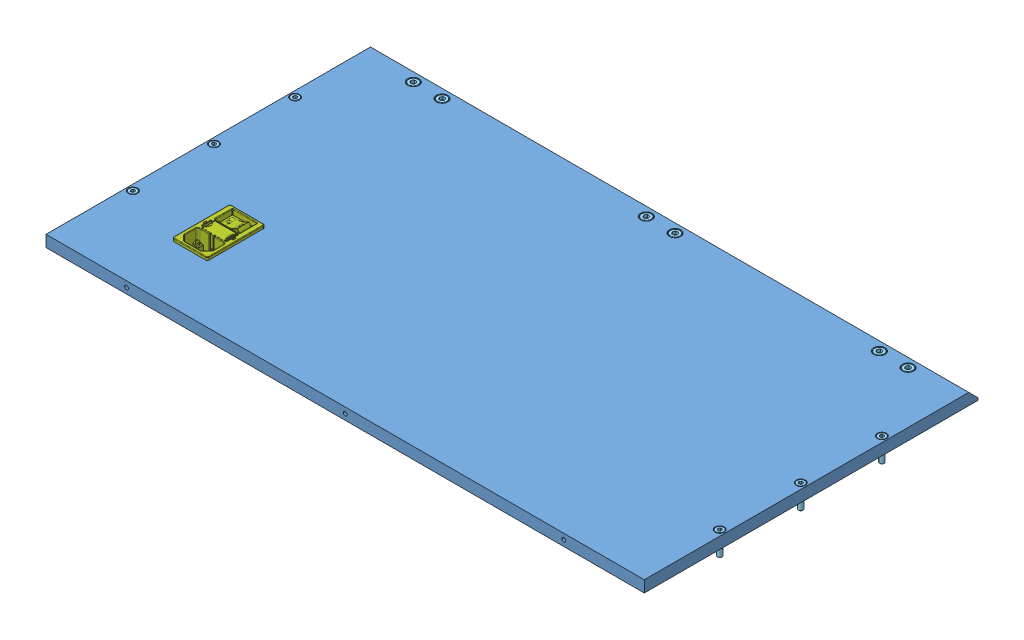
SolidWorks assembly Housing_back, configuration Default. Lengths in mm.
Overall size (520 63.66 290).
37 component instances, 9 part files, 59 mates.
Components (placement in the parent):
- Housing_back-1: Housing_back [Default] at origin size (520 10 290)
- SHPSNA5-1: SHPSNA5 [Closed] at (223 -4.6 -284.75) x (0 0 -1) z (-1 0 0) size (23.16 23.61 41)
  - SHPSNA5_3-1: SHPSNA5_3 [Default] at origin size (22.6 9.2 41)
  - SHPSNA5_7-1: SHPSNA5_7 [Default] x (-0.41399 -0.910281 0) z (0 0 1) size (5 5 41)
  - SHPSNA5_5-1: SHPSNA5_5 [Default] x (-0.130353 0.991468 0) z (0 0 1) size (22.6 9.2 41)
- SHPSNA5-2: SHPSNA5 [Closed] at (20.5 -4.6 -284.75) x (0 0 -1) z (-1 0 0) size (23.16 23.61 41)
  - SHPSNA5_3-1: SHPSNA5_3 [Default] at origin size (22.6 9.2 41)
  - SHPSNA5_7-1: SHPSNA5_7 [Default] x (-0.41399 -0.910281 0) z (0 0 1) size (5 5 41)
  - SHPSNA5_5-1: SHPSNA5_5 [Default] x (-0.130353 0.991468 0) z (0 0 1) size (22.6 9.2 41)
- SHPSNA5-3: SHPSNA5 [Closed] at (-182 -4.6 -284.75) x (0 0 -1) z (-1 0 0) size (23.16 23.61 41)
  - SHPSNA5_3-1: SHPSNA5_3 [Default] at origin size (22.6 9.2 41)
  - SHPSNA5_7-1: SHPSNA5_7 [Default] x (-0.41399 -0.910281 0) z (0 0 1) size (5 5 41)
  - SHPSNA5_5-1: SHPSNA5_5 [Default] x (-0.130353 0.991468 0) z (0 0 1) size (22.6 9.2 41)
- socket head cap screw_iso-2: socket head cap screw_iso [ISO 4762 M5 x 10 - 10N] at (-215 10 -274.25) x (0 -1 0) z (0 0 1) size (15 8.5 8.5)
- socket head cap screw_iso-3: socket head cap screw_iso [ISO 4762 M5 x 10 - 10N] at (-190 10 -274.25) x (0 -1 0) z (0 0 1) size (15 8.5 8.5)
- socket head cap screw_iso-4: socket head cap screw_iso [ISO 4762 M5 x 10 - 10N] at (-12.5 10 -274.25) x (0 -1 0) z (0 0 1) size (15 8.5 8.5)
- socket head cap screw_iso-5: socket head cap screw_iso [ISO 4762 M5 x 10 - 10N] at (12.5 10 -274.25) x (0 -1 0) z (0 0 1) size (15 8.5 8.5)
- socket head cap screw_iso-6: socket head cap screw_iso [ISO 4762 M5 x 10 - 10N] at (190 10 -274.25) x (0 -1 0) z (0 0 1) size (15 8.5 8.5)
- socket head cap screw_iso-7: socket head cap screw_iso [ISO 4762 M5 x 10 - 10N] at (215 10 -274.25) x (0 -1 0) z (0 0 1) size (15 8.5 8.5)
- hex thin nut gradeb_iso-2: hex thin nut gradeb_iso [ISO - 4036 - M5 - N] at (215 -4.7 -274.25) x (1 0 0) z (0 -1 0) size (8 9.24 2.7)
- hex thin nut gradeb_iso-3: hex thin nut gradeb_iso [ISO - 4036 - M5 - N] at (190 -4.7 -274.25) x (1 0 0) z (0 -1 0) size (8 9.24 2.7)
- hex thin nut gradeb_iso-4: hex thin nut gradeb_iso [ISO - 4036 - M5 - N] at (12.5 -4.7 -274.25) x (1 0 0) z (0 -1 0) size (8 9.24 2.7)
- hex thin nut gradeb_iso-5: hex thin nut gradeb_iso [ISO - 4036 - M5 - N] at (-12.5 -4.7 -274.25) x (1 0 0) z (0 -1 0) size (8 9.24 2.7)
- hex thin nut gradeb_iso-6: hex thin nut gradeb_iso [ISO - 4036 - M5 - N] at (-190 -4.7 -274.25) x (1 0 0) z (0 -1 0) size (8 9.24 2.7)
- hex thin nut gradeb_iso-7: hex thin nut gradeb_iso [ISO - 4036 - M5 - N] at (-215 -4.7 -274.25) x (1 0 0) z (0 -1 0) size (8 9.24 2.7)
- socket head cap screw_iso-9: socket head cap screw_iso [ISO 4762 M4 x 16 - 16N] at (-255 10 -211.5) x (0 -1 0) z (0 0 1) size (20 7 7)
- socket head cap screw_iso-10: socket head cap screw_iso [ISO 4762 M4 x 16 - 16N] at (-255 10 -141) x (0 -1 0) z (0 0 1) size (20 7 7)
- socket head cap screw_iso-11: socket head cap screw_iso [ISO 4762 M4 x 16 - 16N] at (-255 10 -70.5) x (0 -1 0) z (0 0 1) size (20 7 7)
- socket head cap screw_iso-12: socket head cap screw_iso [ISO 4762 M4 x 16 - 16N] at (255 10 -70.5) x (0 -1 0) z (0 0 1) size (20 7 7)
- socket head cap screw_iso-13: socket head cap screw_iso [ISO 4762 M4 x 16 - 16N] at (255 10 -211.5) x (0 -1 0) z (0 0 1) size (20 7 7)
- socket head cap screw_iso-14: socket head cap screw_iso [ISO 4762 M4 x 16 - 16N] at (255 10 -141) x (0 -1 0) z (0 0 1) size (20 7 7)
- KMF1.1291.11-1: KMF1.1291.11 [Default] at (-185 10 -60.7) x (-1 0 0) z (0 -1 0) size (31.8 50 43.41)
- CUS-150M-F-1: CUS-150M-F [Default] at (-121.4398 -2.8109 -148.4745) x (0.999999 0 0.001586) z (0.001586 0 -0.999999) size (116.08 50.7 64.1)
- pan head cross recess screw_iso-1: pan head cross recess screw_iso [ISO 7045 - M4 x 6 - Z - 6N] at (-210 -4.3 -140) x (0 1 0) z (-0.546944 0 0.837169) size (9.02 8 8)
- pan head cross recess screw_iso-2: pan head cross recess screw_iso [ISO 7045 - M4 x 6 - Z - 6N] at (-210 -4.3 -175) x (0 1 0) z (-0.546944 0 0.837169) size (9.02 8 8)
- pan head cross recess screw_iso-3: pan head cross recess screw_iso [ISO 7045 - M4 x 6 - Z - 6N] at (-99.4 -4.3 -140) x (0 1 0) z (-0.546944 0 0.837169) size (9.02 8 8)
- pan head cross recess screw_iso-4: pan head cross recess screw_iso [ISO 7045 - M4 x 6 - Z - 6N] at (-99.4 -4.3 -175) x (0 1 0) z (-0.546944 0 0.837169) size (9.02 8 8)
Mates (geometry in assembly coordinates):
- Coincident1: coincident anti-aligned: plane of Housing_back-1 through (0 0 0) normal (0 -1 0); plane of SHPSNA5-1/SHPSNA5_3-1 through (182 0 -266.75) normal (0 1 0)
- Coincident3: coincident anti-aligned: plane of Housing_back-1 through (0 0 0) normal (0 -1 0); plane of SHPSNA5-2/SHPSNA5_3-1 through (-20.5 0 -266.75) normal (0 1 0)
- Coincident4: coincident anti-aligned: plane of Housing_back-1 through (0 0 0) normal (0 -1 0); plane of SHPSNA5-3/SHPSNA5_3-1 through (-223 0 -266.75) normal (0 1 0)
- Concentric1: concentric aligned: cylinder of Housing_back-1 through (-215 10 -274.25) axis (0 1 0) radius 5; cylinder of SHPSNA5-3/SHPSNA5_3-1 through (-215 -2 -274.25) axis (0 1 0) radius 2.75
- Concentric2: concentric aligned: cylinder of Housing_back-1 through (-190 10 -274.25) axis (0 1 0) radius 5; cylinder of SHPSNA5-3/SHPSNA5_3-1 through (-190 -2 -274.25) axis (0 1 0) radius 2.75
- Concentric3: concentric aligned: cylinder of Housing_back-1 through (-12.5 10 -274.25) axis (0 1 0) radius 5; cylinder of SHPSNA5-2/SHPSNA5_3-1 through (-12.5 -2 -274.25) axis (0 1 0) radius 2.75
- Concentric4: concentric aligned: cylinder of Housing_back-1 through (12.5 10 -274.25) axis (0 1 0) radius 5; cylinder of SHPSNA5-2/SHPSNA5_3-1 through (12.5 -2 -274.25) axis (0 1 0) radius 2.75
- Concentric5: concentric aligned: cylinder of Housing_back-1 through (190 10 -274.25) axis (0 1 0) radius 5; cylinder of SHPSNA5-1/SHPSNA5_3-1 through (190 -2 -274.25) axis (0 1 0) radius 2.75
- Concentric6: concentric aligned: cylinder of Housing_back-1 through (215 10 -274.25) axis (0 1 0) radius 5; cylinder of SHPSNA5-1/SHPSNA5_3-1 through (215 -2 -274.25) axis (0 1 0) radius 2.75
- Concentric7: concentric aligned: cylinder of Housing_back-1 through (-215 10 -274.25) axis (0 1 0) radius 2.75; cylinder of socket head cap screw_iso-2 through (-215 41.75 -274.25) axis (0 1 0) radius 4.25
- Coincident5: coincident anti-aligned: plane of Housing_back-1 through (-212.25 5 -274.25) normal (0 1 0); plane of socket head cap screw_iso-2 through (-210.75 5 -274.25) normal (0 -1 0)
- Concentric8: concentric aligned: cylinder of Housing_back-1 through (-190 10 -274.25) axis (0 1 0) radius 5; cylinder of socket head cap screw_iso-3 through (-190 41.75 -274.25) axis (0 1 0) radius 4.25
- Coincident6: coincident anti-aligned: plane of Housing_back-1 through (-187.25 5 -274.25) normal (0 1 0); plane of socket head cap screw_iso-3 through (-185.75 5 -274.25) normal (0 -1 0)
- Concentric9: concentric aligned: cylinder of Housing_back-1 through (-12.5 10 -274.25) axis (0 1 0) radius 2.75; cylinder of socket head cap screw_iso-4 through (-12.5 41.75 -274.25) axis (0 1 0) radius 4.25
- Coincident7: coincident anti-aligned: plane of Housing_back-1 through (-9.75 5 -274.25) normal (0 1 0); plane of socket head cap screw_iso-4 through (-8.25 5 -274.25) normal (0 -1 0)
- Concentric10: concentric aligned: cylinder of Housing_back-1 through (12.5 10 -274.25) axis (0 1 0) radius 2.75; cylinder of socket head cap screw_iso-5 through (12.5 41.75 -274.25) axis (0 1 0) radius 4.25
- Coincident8: coincident anti-aligned: plane of Housing_back-1 through (15.25 5 -274.25) normal (0 1 0); plane of socket head cap screw_iso-5 through (16.75 5 -274.25) normal (0 -1 0)
- Concentric11: concentric aligned: cylinder of Housing_back-1 through (190 10 -274.25) axis (0 1 0) radius 2.75; cylinder of socket head cap screw_iso-6 through (190 41.75 -274.25) axis (0 1 0) radius 4.25
- Coincident9: coincident anti-aligned: plane of Housing_back-1 through (192.75 5 -274.25) normal (0 1 0); plane of socket head cap screw_iso-6 through (194.25 5 -274.25) normal (0 -1 0)
- Concentric12: concentric aligned: cylinder of Housing_back-1 through (215 10 -274.25) axis (0 1 0) radius 2.75; cylinder of socket head cap screw_iso-7 through (215 41.75 -274.25) axis (0 1 0) radius 4.25
- Coincident10: coincident anti-aligned: plane of Housing_back-1 through (217.75 5 -274.25) normal (0 1 0); plane of socket head cap screw_iso-7 through (219.25 5 -274.25) normal (0 -1 0)
- Concentric13: concentric anti-aligned: cylinder of SHPSNA5-1/SHPSNA5_3-1 through (215 -2 -274.25) axis (0 1 0) radius 2.75; cylinder of hex thin nut gradeb_iso-2 through (215 20.3375 -274.25) axis (0 -1 0) radius 2.5
- Coincident11: coincident anti-aligned: plane of SHPSNA5-1/SHPSNA5_3-1 through (182 -2 -280.9553) normal (0 -1 0); plane of hex thin nut gradeb_iso-2 through (207 -2 -274.25) normal (0 1 0)
- Concentric14: concentric anti-aligned: cylinder of SHPSNA5-1/SHPSNA5_3-1 through (190 -2 -274.25) axis (0 1 0) radius 2.75; cylinder of hex thin nut gradeb_iso-3 through (190 20.3375 -274.25) axis (0 -1 0) radius 2.5
- Coincident12: coincident anti-aligned: plane of SHPSNA5-1/SHPSNA5_3-1 through (182 -2 -280.9553) normal (0 -1 0); plane of hex thin nut gradeb_iso-3 through (182 -2 -274.25) normal (0 1 0)
- Concentric15: concentric anti-aligned: cylinder of SHPSNA5-2/SHPSNA5_3-1 through (12.5 -2 -274.25) axis (0 1 0) radius 2.75; cylinder of hex thin nut gradeb_iso-4 through (12.5 20.3375 -274.25) axis (0 -1 0) radius 2.5
- Coincident13: coincident anti-aligned: plane of SHPSNA5-2/SHPSNA5_3-1 through (-20.5 -2 -280.9553) normal (0 -1 0); plane of hex thin nut gradeb_iso-4 through (4.5 -2 -274.25) normal (0 1 0)
- Concentric16: concentric anti-aligned: cylinder of SHPSNA5-2/SHPSNA5_3-1 through (-12.5 -2 -274.25) axis (0 1 0) radius 2.75; cylinder of hex thin nut gradeb_iso-5 through (-12.5 20.3375 -274.25) axis (0 -1 0) radius 2.5
- Coincident14: coincident anti-aligned: plane of SHPSNA5-2/SHPSNA5_3-1 through (-20.5 -2 -280.9553) normal (0 -1 0); plane of hex thin nut gradeb_iso-5 through (-20.5 -2 -274.25) normal (0 1 0)
- Concentric17: concentric anti-aligned: cylinder of SHPSNA5-3/SHPSNA5_3-1 through (-190 -2 -274.25) axis (0 1 0) radius 2.75; cylinder of hex thin nut gradeb_iso-6 through (-190 20.3375 -274.25) axis (0 -1 0) radius 2.5
- Coincident15: coincident anti-aligned: plane of SHPSNA5-3/SHPSNA5_3-1 through (-223 -2 -280.9553) normal (0 -1 0); plane of hex thin nut gradeb_iso-6 through (-198 -2 -274.25) normal (0 1 0)
- Concentric18: concentric anti-aligned: cylinder of SHPSNA5-3/SHPSNA5_3-1 through (-215 -2 -274.25) axis (0 1 0) radius 2.75; cylinder of hex thin nut gradeb_iso-7 through (-215 20.3375 -274.25) axis (0 -1 0) radius 2.5
- Coincident16: coincident anti-aligned: plane of SHPSNA5-3/SHPSNA5_3-1 through (-223 -2 -280.9553) normal (0 -1 0); plane of hex thin nut gradeb_iso-7 through (-223 -2 -274.25) normal (0 1 0)
- Concentric19: concentric aligned: cylinder of Housing_back-1 through (-255 10 -211.5) axis (0 1 0) radius 2.25; cylinder of socket head cap screw_iso-9 through (-255 41.75 -211.5) axis (0 1 0) radius 3.5
- Coincident17: coincident anti-aligned: plane of Housing_back-1 through (-252.75 6 -211.5) normal (0 1 0); plane of socket head cap screw_iso-9 through (-251.5 6 -211.5) normal (0 -1 0)
- Concentric20: concentric aligned: cylinder of Housing_back-1 through (-255 10 -141) axis (0 1 0) radius 2.25; cylinder of socket head cap screw_iso-10 through (-255 41.75 -141) axis (0 1 0) radius 3.5
- Coincident18: coincident anti-aligned: plane of Housing_back-1 through (-252.75 6 -141) normal (0 1 0); plane of socket head cap screw_iso-10 through (-251.5 6 -141) normal (0 -1 0)
- Concentric21: concentric aligned: cylinder of Housing_back-1 through (-255 10 -70.5) axis (0 1 0) radius 4; cylinder of socket head cap screw_iso-11 through (-255 41.75 -70.5) axis (0 1 0) radius 3.5
- Coincident19: coincident anti-aligned: plane of Housing_back-1 through (-252.75 6 -70.5) normal (0 1 0); plane of socket head cap screw_iso-11 through (-251.5 6 -70.5) normal (0 -1 0)
- Concentric22: concentric aligned: cylinder of Housing_back-1 through (255 10 -70.5) axis (0 1 0) radius 2.25; cylinder of socket head cap screw_iso-12 through (255 41.75 -70.5) axis (0 1 0) radius 3.5
- Coincident20: coincident anti-aligned: plane of Housing_back-1 through (257.25 6 -70.5) normal (0 1 0); plane of socket head cap screw_iso-12 through (258.5 6 -70.5) normal (0 -1 0)
- Concentric23: concentric aligned: cylinder of Housing_back-1 through (255 10 -211.5) axis (0 1 0) radius 2.25; cylinder of socket head cap screw_iso-13 through (255 41.75 -211.5) axis (0 1 0) radius 3.5
- Coincident21: coincident anti-aligned: plane of Housing_back-1 through (257.25 6 -211.5) normal (0 1 0); plane of socket head cap screw_iso-13 through (258.5 6 -211.5) normal (0 -1 0)
- Concentric24: concentric aligned: cylinder of Housing_back-1 through (255 10 -141) axis (0 1 0) radius 2.25; cylinder of socket head cap screw_iso-14 through (255 41.75 -141) axis (0 1 0) radius 3.5
- Coincident22: coincident anti-aligned: plane of Housing_back-1 through (257.25 6 -141) normal (0 1 0); plane of socket head cap screw_iso-14 through (258.5 6 -141) normal (0 -1 0)
- Width2: width anti-aligned: plane of KMF1.1291.11-1 through (-199.25 10 -52.1) normal (-1 0 0); plane of KMF1.1291.11-1 through (-170.75 10 -52.1) normal (1 0 0); plane of Housing_back-1 through (-199.75 0 -99.25) normal (1 0 0); plane of Housing_back-1 through (-170.25 0 -99.25) normal (-1 0 0)
- Width3: width anti-aligned: plane of KMF1.1291.11-1 through (-198.4 10 -98.75) normal (0 0 -1); plane of KMF1.1291.11-1 through (-171.6 10 -51.25) normal (0 0 1); plane of Housing_back-1 through (-199.75 0 -99.25) normal (0 0 1); plane of Housing_back-1 through (-199.75 0 -50.75) normal (0 0 -1)
- Coincident23: coincident anti-aligned: plane of Housing_back-1 through (0 10 0) normal (0 1 0); plane of KMF1.1291.11-1 through (-198.75 10 -98.5) normal (0 -1 0)
- Coincident24: coincident anti-aligned: plane of Housing_back-1 through (0 0 0) normal (0 -1 0); plane of CUS-150M-F-1 through (-96.7 0 -125.6) normal (0 1 0)
- Concentric25: concentric aligned: cylinder of Housing_back-1 through (-210 0 -140) axis (0 -1 0) radius 1.65; cylinder of pan head cross recess screw_iso-1 through (-210 -29.7 -140) axis (0 -1 0) radius 2
- Concentric26: concentric aligned: cylinder of Housing_back-1 through (-210 0 -175) axis (0 -1 0) radius 1.65; cylinder of pan head cross recess screw_iso-2 through (-210 -29.7 -175) axis (0 -1 0) radius 2
- Concentric27: concentric aligned: cylinder of Housing_back-1 through (-99.4 0 -140) axis (0 -1 0) radius 1.65; cylinder of pan head cross recess screw_iso-3 through (-99.4 -29.7 -140) axis (0 -1 0) radius 2
- Concentric28: concentric aligned: cylinder of Housing_back-1 through (-99.4 0 -175) axis (0 -1 0) radius 1.65; cylinder of pan head cross recess screw_iso-4 through (-99.4 -29.7 -175) axis (0 -1 0) radius 2
- Distance2: distance = 1.2 mm anti-aligned: plane of pan head cross recess screw_iso-2 through (-211.6743 -1.2 -176.0939) normal (0 1 0); plane of Housing_back-1 through (0 0 0) normal (0 -1 0)
- Distance3: distance = 1.2 mm anti-aligned: plane of pan head cross recess screw_iso-1 through (-211.6743 -1.2 -141.0939) normal (0 1 0); plane of Housing_back-1 through (0 0 0) normal (0 -1 0)
- Distance4: distance = 1.2 mm anti-aligned: plane of pan head cross recess screw_iso-3 through (-101.0743 -1.2 -141.0939) normal (0 1 0); plane of Housing_back-1 through (0 0 0) normal (0 -1 0)
- Distance5: distance = 1.2 mm anti-aligned: plane of pan head cross recess screw_iso-4 through (-101.0743 -1.2 -176.0939) normal (0 1 0); plane of Housing_back-1 through (0 0 0) normal (0 -1 0)
- Concentric29: concentric anti-aligned: line of CUS-150M-F-1 through (-99.4 -1.26 -175) axis (0 1 0); cylinder of pan head cross recess screw_iso-4 through (-99.4 -29.7 -175) axis (0 -1 0) radius 2
- Concentric30: concentric anti-aligned: line of CUS-150M-F-1 through (-210 -1.26 -140) axis (0 1 0); cylinder of pan head cross recess screw_iso-1 through (-210 -29.7 -140) axis (0 -1 0) radius 2
